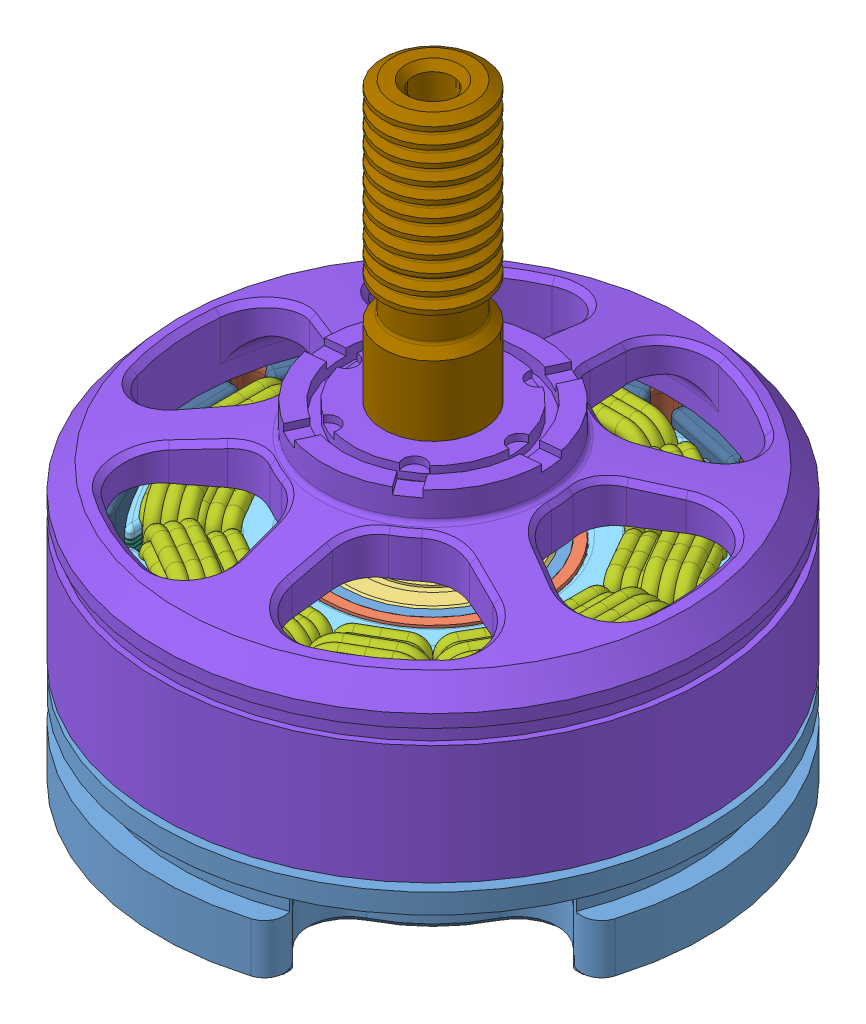
SolidWorks assembly F40, configuration CCW. Lengths in mm.
Overall size (36.43 31.7 36.43).
59 component instances, 12 part files, 5 mates.
Components (placement in the parent):
- Stator^F40-1: Stator^F40 [Défaut] at origin size (27.5 13.15 27.5) (virtual)
  - Stator Housing^Stator_F40-1: Stator Housing^Stator_F40 [Défaut] at origin size (27.5 11.8 27.5) (virtual)
  - Stator Sleeve^Stator_F40-1: Stator Sleeve^Stator_F40 [Défaut] at (0 6.8 0) x (0.969213 0 -0.246225) z (0.246225 0 0.969213) size (11 5 11) (virtual)
  - Stator Bearing A^Stator_F40-1: Stator Bearing A^Stator_F40 [7804K126] at (0 9.8 0) x (0.986636 0 -0.162941) z (0 1 0) size (9 9 4) (virtual)
  - Stator Bearing B^Stator_F40-1: Stator Bearing B^Stator_F40 [7804K126] at (0 2.95 0) x (0.998438 0 -0.055866) z (0 1 0) size (9 9 3.5) (virtual)
  - Stator Core^Stator_F40-2: Stator Core^Stator_F40 [Défaut] at (0 7.3 0) size (22 7.7 22) (virtual)
    - Epoxy Plate^Stator Core_Stator_F40-1: Epoxy Plate^Stator Core_Stator_F40 [Défaut] x (-1 0 0) z (0 0 1) size (22 0.52 22) (virtual)
    - Stator Plate^Stator Core_Stator_F40-1: Stator Plate^Stator Core_Stator_F40 [Défaut] at origin size (22 0.2 22) (virtual)
    - Stator Plate^Stator Core_Stator_F40-21: Stator Plate^Stator Core_Stator_F40 [Défaut] at (0 0.2 0) size (22 0.2 22) (virtual)
    - Stator Plate^Stator Core_Stator_F40-22: Stator Plate^Stator Core_Stator_F40 [Défaut] at (0 0.4 0) size (22 0.2 22) (virtual)
    - Stator Plate^Stator Core_Stator_F40-23: Stator Plate^Stator Core_Stator_F40 [Défaut] at (0 0.6 0) size (22 0.2 22) (virtual)
    - Stator Plate^Stator Core_Stator_F40-24: Stator Plate^Stator Core_Stator_F40 [Défaut] at (0 0.8 0) size (22 0.2 22) (virtual)
    - Stator Plate^Stator Core_Stator_F40-25: Stator Plate^Stator Core_Stator_F40 [Défaut] at (0 1 0) size (22 0.2 22) (virtual)
    - Stator Plate^Stator Core_Stator_F40-26: Stator Plate^Stator Core_Stator_F40 [Défaut] at (0 1.2 0) size (22 0.2 22) (virtual)
    - Stator Plate^Stator Core_Stator_F40-27: Stator Plate^Stator Core_Stator_F40 [Défaut] at (0 1.4 0) size (22 0.2 22) (virtual)
    - Stator Plate^Stator Core_Stator_F40-28: Stator Plate^Stator Core_Stator_F40 [Défaut] at (0 1.6 0) size (22 0.2 22) (virtual)
    - Stator Plate^Stator Core_Stator_F40-29: Stator Plate^Stator Core_Stator_F40 [Défaut] at (0 1.8 0) size (22 0.2 22) (virtual)
    - Stator Plate^Stator Core_Stator_F40-30: Stator Plate^Stator Core_Stator_F40 [Défaut] at (0 2 0) size (22 0.2 22) (virtual)
    - Stator Plate^Stator Core_Stator_F40-31: Stator Plate^Stator Core_Stator_F40 [Défaut] at (0 2.2 0) size (22 0.2 22) (virtual)
    - Stator Plate^Stator Core_Stator_F40-32: Stator Plate^Stator Core_Stator_F40 [Défaut] at (0 2.4 0) size (22 0.2 22) (virtual)
    - Stator Plate^Stator Core_Stator_F40-33: Stator Plate^Stator Core_Stator_F40 [Défaut] at (0 2.6 0) size (22 0.2 22) (virtual)
    - Stator Plate^Stator Core_Stator_F40-34: Stator Plate^Stator Core_Stator_F40 [Défaut] at (0 2.8 0) size (22 0.2 22) (virtual)
    - Stator Plate^Stator Core_Stator_F40-35: Stator Plate^Stator Core_Stator_F40 [Défaut] at (0 3 0) size (22 0.2 22) (virtual)
    - Stator Plate^Stator Core_Stator_F40-36: Stator Plate^Stator Core_Stator_F40 [Défaut] at (0 3.2 0) size (22 0.2 22) (virtual)
    - Stator Plate^Stator Core_Stator_F40-37: Stator Plate^Stator Core_Stator_F40 [Défaut] at (0 3.4 0) size (22 0.2 22) (virtual)
    - Stator Plate^Stator Core_Stator_F40-38: Stator Plate^Stator Core_Stator_F40 [Défaut] at (0 3.6 0) size (22 0.2 22) (virtual)
    - Stator Plate^Stator Core_Stator_F40-39: Stator Plate^Stator Core_Stator_F40 [Défaut] at (0 3.8 0) size (22 0.2 22) (virtual)
    - Epoxy Plate^Stator Core_Stator_F40-2: Epoxy Plate^Stator Core_Stator_F40 [Défaut] at (0 4 0) size (22 0.52 22) (virtual)
    - Stator Coil^Stator Core_Stator_F40-1: Stator Coil^Stator Core_Stator_F40 [Défaut] at origin size (3.75 7.7 4.95) (virtual)
    - Stator Coil^Stator Core_Stator_F40-2: Stator Coil^Stator Core_Stator_F40 [Défaut] x (0.866025 0 -0.5) z (0.5 0 0.866025) size (3.75 7.7 4.95) (virtual)
    - Stator Coil^Stator Core_Stator_F40-3: Stator Coil^Stator Core_Stator_F40 [Défaut] x (0.5 0 -0.866025) z (0.866025 0 0.5) size (3.75 7.7 4.95) (virtual)
    - Stator Coil^Stator Core_Stator_F40-4: Stator Coil^Stator Core_Stator_F40 [Défaut] x (0 0 -1) z (1 0 0) size (3.75 7.7 4.95) (virtual)
    - Stator Coil^Stator Core_Stator_F40-5: Stator Coil^Stator Core_Stator_F40 [Défaut] x (-0.5 0 -0.866025) z (0.866025 0 -0.5) size (3.75 7.7 4.95) (virtual)
    - Stator Coil^Stator Core_Stator_F40-6: Stator Coil^Stator Core_Stator_F40 [Défaut] x (-0.866025 0 -0.5) z (0.5 0 -0.866025) size (3.75 7.7 4.95) (virtual)
    - Stator Coil^Stator Core_Stator_F40-7: Stator Coil^Stator Core_Stator_F40 [Défaut] x (-1 0 0) z (0 0 -1) size (3.75 7.7 4.95) (virtual)
    - Stator Coil^Stator Core_Stator_F40-8: Stator Coil^Stator Core_Stator_F40 [Défaut] x (-0.866025 0 0.5) z (-0.5 0 -0.866025) size (3.75 7.7 4.95) (virtual)
    - Stator Coil^Stator Core_Stator_F40-9: Stator Coil^Stator Core_Stator_F40 [Défaut] x (-0.5 0 0.866025) z (-0.866025 0 -0.5) size (3.75 7.7 4.95) (virtual)
    - Stator Coil^Stator Core_Stator_F40-10: Stator Coil^Stator Core_Stator_F40 [Défaut] x (0 0 1) z (-1 0 0) size (3.75 7.7 4.95) (virtual)
    - Stator Coil^Stator Core_Stator_F40-11: Stator Coil^Stator Core_Stator_F40 [Défaut] x (0.5 0 0.866025) z (-0.866025 0 0.5) size (3.75 7.7 4.95) (virtual)
    - Stator Coil^Stator Core_Stator_F40-12: Stator Coil^Stator Core_Stator_F40 [Défaut] x (0.866025 0 0.5) z (-0.5 0 0.866025) size (3.75 7.7 4.95) (virtual)
- Rotor^F40-1: Rotor^F40 [CW] at (0 6.4 0) x (-0.909769 0 -0.415114) z (0.415114 0 -0.909769) size (27.5 31.7 27.5) (virtual)
  - Rotor Housing^Rotor_F40-1: Rotor Housing^Rotor_F40 [Défaut] at origin size (27.5 11.3 27.5) (virtual)
  - Shaft^Rotor_F40-1: Shaft^Rotor_F40 [CW] at (0 -6.4 0) size (7 31.7 7) (virtual)
  - Rotor Magnet^Rotor_F40-1: Rotor Magnet^Rotor_F40 [Défaut] at (-12.0853 2.9 0) x (0 0 -1) z (1 0 0) size (4 5 1.5) (virtual)
  - Rotor Magnet^Rotor_F40-15: Rotor Magnet^Rotor_F40 [Défaut] at (-10.8884 2.9 -5.2436) x (0.433884 0 -0.900969) z (0.900969 0 0.433884) size (4 5 1.5) (virtual)
  - Rotor Magnet^Rotor_F40-16: Rotor Magnet^Rotor_F40 [Défaut] at (-7.535 2.9 -9.4486) x (0.781831 0 -0.62349) z (0.62349 0 0.781831) size (4 5 1.5) (virtual)
  - Rotor Magnet^Rotor_F40-17: Rotor Magnet^Rotor_F40 [Défaut] at (-2.6892 2.9 -11.7822) x (0.974928 0 -0.222521) z (0.222521 0 0.974928) size (4 5 1.5) (virtual)
  - Rotor Magnet^Rotor_F40-18: Rotor Magnet^Rotor_F40 [Défaut] at (2.6892 2.9 -11.7822) x (0.974928 0 0.222521) z (-0.222521 0 0.974928) size (4 5 1.5) (virtual)
  - Rotor Magnet^Rotor_F40-19: Rotor Magnet^Rotor_F40 [Défaut] at (7.535 2.9 -9.4486) x (0.781831 0 0.62349) z (-0.62349 0 0.781831) size (4 5 1.5) (virtual)
  - Rotor Magnet^Rotor_F40-20: Rotor Magnet^Rotor_F40 [Défaut] at (10.8884 2.9 -5.2436) x (0.433884 0 0.900969) z (-0.900969 0 0.433884) size (4 5 1.5) (virtual)
  - Rotor Magnet^Rotor_F40-21: Rotor Magnet^Rotor_F40 [Défaut] at (12.0853 2.9 0) x (0 0 1) z (-1 0 0) size (4 5 1.5) (virtual)
  - Rotor Magnet^Rotor_F40-22: Rotor Magnet^Rotor_F40 [Défaut] at (10.8884 2.9 5.2436) x (-0.433884 0 0.900969) z (-0.900969 0 -0.433884) size (4 5 1.5) (virtual)
  - Rotor Magnet^Rotor_F40-23: Rotor Magnet^Rotor_F40 [Défaut] at (7.535 2.9 9.4486) x (-0.781831 0 0.62349) z (-0.62349 0 -0.781831) size (4 5 1.5) (virtual)
  - Rotor Magnet^Rotor_F40-24: Rotor Magnet^Rotor_F40 [Défaut] at (2.6892 2.9 11.7822) x (-0.974928 0 0.222521) z (-0.222521 0 -0.974928) size (4 5 1.5) (virtual)
  - Rotor Magnet^Rotor_F40-25: Rotor Magnet^Rotor_F40 [Défaut] at (-2.6892 2.9 11.7822) x (-0.974928 0 -0.222521) z (0.222521 0 -0.974928) size (4 5 1.5) (virtual)
  - Rotor Magnet^Rotor_F40-26: Rotor Magnet^Rotor_F40 [Défaut] at (-7.535 2.9 9.4486) x (-0.781831 0 -0.62349) z (0.62349 0 -0.781831) size (4 5 1.5) (virtual)
  - Rotor Magnet^Rotor_F40-27: Rotor Magnet^Rotor_F40 [Défaut] at (-10.8884 2.9 5.2436) x (-0.433884 0 -0.900969) z (0.900969 0 -0.433884) size (4 5 1.5) (virtual)
  - Epoxy Glue^Rotor_F40-1: Epoxy Glue^Rotor_F40 [Défaut] at (0 5.5 0) x (-1 0 0) z (0 -1 0) size (25.9 25.9 5.31) (virtual)
- Circlip^F40-1: Circlip^F40 [98541A111] at (0 0.8 0) x (0 -1 0) z (-0.503235 0 0.86415) size (0.4 6.1 4.7) (virtual)
Mates (geometry in assembly coordinates):
- Coaxiale1: concentric anti-aligned: cylinder of Rotor^F40-1/Shaft^Rotor_F40-1 through (0 -309.2183 0) axis (0 -1 0) radius 1.95; cylinder of ? through (0 -10.9166 0) axis (0 1 0) radius 2
- Distance1: distance = 17.7 mm anti-aligned: plane of Rotor^F40-1/Rotor Housing^Rotor_F40-1 through (0 17.7 0) normal (0 1 0); plane of Stator^F40-1/Stator Housing^Stator_F40-1 through (0 0 -5.6928) normal (0 -1 0)
- Coaxiale2: concentric anti-aligned: cylinder of Rotor^F40-1/Shaft^Rotor_F40-1 through (0 -309.2183 0) axis (0 -1 0) radius 1.7; cylinder of Circlip^F40-1 through (0 0.6 0) axis (0 1 0) radius 1.7
- Tangent1: tangent: torus of Rotor^F40-1/Shaft^Rotor_F40-1; plane of Circlip^F40-1 through (0 0.6 0) normal (0 -1 0)
- Coaxiale3: concentric anti-aligned: cylinder of Stator^F40-1/Stator Bearing A^Stator_F40-1 through (0 11.8 0) axis (0 1 0) radius 2; cylinder of Rotor^F40-1/Shaft^Rotor_F40-1 through (0 -309.2183 0) axis (0 -1 0) radius 2.5
